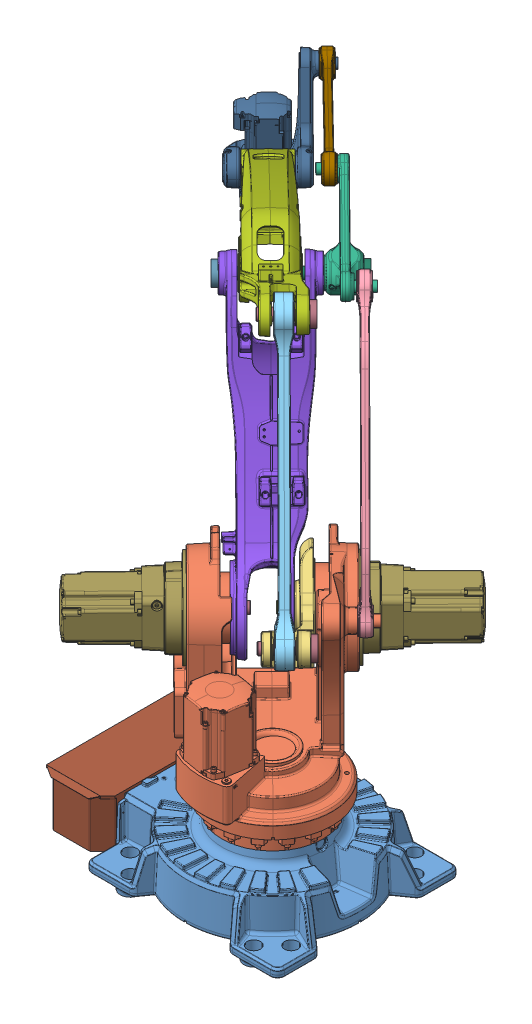
SolidWorks assembly 装配体, configuration 默认. Lengths in mm.
Overall size (188.36 192.9 189.31).
24 component instances, 20 part files, 53 mates.
Components (placement in the parent):
- 111-1: 111 [Default] at (31.9169 -93.0773 0.0393) size (77.8 26.1 72.28)
- 222-1: 222 [Default] at (108.2572 -470.9107 80.6307) x (-0.711585 0 -0.7026) z (0.7026 0 -0.711585) size (72.42 79.23 57.6)
- 333-1: 333 [Default] at (-54.6427 48.8539 -123.2904) x (0.674502 0.318604 0.665987) z (-0.7026 0 0.711585) size (59.48 34.02 15.46)
- 444-1: 444 [Default] at (139.3919 -302.9342 96.1752) x (-0.640122 -0.436772 -0.63204) z (0.7026 0 -0.711585) size (13.8 104.1 4.57)
- 555-1: 555 [Default] at (149.2261 -292.6873 136.4449) x (0.640122 0.436772 0.63204) z (-0.7026 0 0.711585) size (12.5 107 6.85)
- 666-1: 666 [Default] at (-33.4489 78.7584 -68.0821) x (0.700774 -0.173648 0.691926) z (-0.7026 0 0.711585) size (58.22 29.07 16.9)
- 777-2: 777 [Default] at (110.2288 184.9276 106.6261) x (0.7026 0 -0.711585) z (0.674502 0.318604 0.665987) size (19.78 28.14 154.01)
- 888-1: 888 [Default] at (110.474 -208.6533 84.8633) x (-0.640122 -0.436772 -0.63204) z (0.7026 0 -0.711585) size (35.62 116.33 33.14)
- 999-1: 999 [Default] at (261.0446 326.7026 228.677) x (0.226714 -0.947888 0.223851) z (0.7026 0 -0.711585) size (9.6 112.1 5.52)
- 100-1: 100 [默认] at (759.4438 355.8144 743.7493) x (0.7026 0 -0.711585) z (0.711585 0 0.7026) size (32.4 48.93 38.5)
- 1111-1: 1111 [Default] at (482.4826 -100.5846 -7.6891) size (25.2 20.1 57.39)
- 电机-1: 电机 [Default] at (107.7654 -470.9107 81.1289) x (-0.711585 0 -0.7026) z (0.7026 0 -0.711585) size (32.5 32.5 40.6)
- 电机-2: 电机 [Default] at (-132.1184 -470.9107 -117.9487) x (0.711585 0 0.7026) z (-0.7026 0 0.711585) size (32.5 32.5 40.6)
- 销轴1-1: 销轴1 [默认] at (22.1458 89.8559 0.7935) x (0.711585 0 0.7026) z (-0.7026 0 0.711585) size (8 8 17)
- 销轴1-2: 销轴1 [默认] at (-7.2775 174.8655 -28.1529) x (0.711585 0 0.7026) z (-0.7026 0 0.711585) size (8 8 17)
- 销轴2-1: 销轴2 [默认] at (-52.0159 162.1213 -36.8071) x (-0.711585 0 -0.7026) z (0.7026 0 -0.711585) size (8 8 13)
- 销轴3-1: 销轴3 [默认] at (-23.4903 162.1213 -65.6974) x (0.711585 0 0.7026) z (-0.7026 0 0.711585) size (8 8 25)
- 销轴1-3: 销轴1 [默认] at (-27.0014 77.1117 -3.3955) x (-0.022337 0.999507 -0.022055) z (0.7026 0 -0.711585) size (8 8 17)
- 销轴4-1: 销轴4 [默认] at (2.6483 77.1117 -33.4244) x (0.711585 0 0.7026) z (-0.7026 0 0.711585) size (8 8 22)
- 零件21-1: 零件21 [默认] at (31.9169 8.1617 0.0393) x (-1 0 0) z (0 1 0)
- 零件22-1: 零件22 [默认] at origin
- 零件23-1: 零件23 [默认] at origin
- 销轴5-1: 销轴5 [默认] at (-113.9156 129.4644 -112.4) x (0.711585 0 0.7026) z (-0.7026 0 0.711585) size (4 4 8.5)
- 销轴5-2: 销轴5 [默认] at (-102.0416 129.4644 -124.4258) x (0.711585 0 0.7026) z (-0.7026 0 0.711585) size (4 4 8.5)
Mates (geometry in assembly coordinates):
- 重合1: coincident anti-aligned: plane of 111-1 through (23.1842 26.4117 0) normal (0 1 0); plane of 222-1 through (18.2811 26.4117 11.9442) normal (0 -1 0)
- 距离4: distance = 6.45 mm aligned: plane of 777-2 through (-7.2775 174.8655 -28.1529) normal (0.7026 0 -0.711585); plane of 555-1 through (-11.8093 174.8655 -23.5632) normal (0.7026 0 -0.711585)
- 距离5: distance = 16.5 mm anti-aligned: plane of 888-1 through (-17.5163 77.1117 -13.0019) normal (0.7026 0 -0.711585); plane of 222-1 through (-29.1092 77.1117 -1.2607) normal (-0.7026 0 0.711585)
- 宽度2: width aligned: plane of 1111-1 through (-37.6535 4.5617 28.3619) normal (0 0 1); plane of 1111-1 through (-37.6535 22.3617 -28.3619) normal (0 0 -1); plane of 111-1 through (-31.711 8.1617 20.8505) normal (0 0.052336 0.99863); plane of 111-1 through (-25.55 8.1617 -20.8505) normal (0 0.052336 -0.99863)
- 同心13: concentric aligned: cylinder of 222-1 through (23.1833 91.1959 -16.5214) axis (0.7026 0 -0.711585) radius 2; cylinder of 444-1 through (19.5298 91.1959 -12.8211) axis (0.7026 0 -0.711585) radius 2.25
- 同心14: concentric aligned: cylinder of 333-1 through (12.5265 89.8559 10.5357) axis (0.7026 0 -0.711585) radius 2; cylinder of 555-1 through (4.4094 89.8559 18.7566) axis (0.7026 0 -0.711585) radius 2.25
- 宽度3: width anti-aligned: plane of 333-1 through (-46.9472 200.689 -62.2977) normal (-0.7026 0 0.711585); plane of 333-1 through (-16.9048 75.3142 -22.3056) normal (0.7026 0 -0.711585); plane of 555-1 through (18.9665 89.8559 4.0134) normal (0.7026 0 -0.711585); plane of 555-1 through (15.0319 89.8559 7.9983) normal (-0.7026 0 0.711585)
- 同心15: concentric aligned: cylinder of 333-1 through (12.5265 89.8559 10.5357) axis (0.7026 0 -0.711585) radius 2; cylinder of 销轴1-1 through (11.6067 89.8559 11.4672) axis (0.7026 0 -0.711585) radius 2
- 重合16: coincident anti-aligned: plane of 333-1 through (28.8056 77.7045 7.3692) normal (0.7026 0 -0.711585); plane of 销轴1-1 through (22.1458 89.8559 0.7935) normal (-0.7026 0 0.711585)
- 同心16: concentric aligned: cylinder of 555-1 through (-24.1632 174.8655 -11.0514) axis (0.7026 0 -0.711585) radius 2.25; cylinder of 777-2 through (-19.7388 174.8655 -15.5324) axis (0.7026 0 -0.711585) radius 2
- 同心17: concentric aligned: cylinder of 777-2 through (-19.7388 174.8655 -15.5324) axis (0.7026 0 -0.711585) radius 2; cylinder of 销轴1-2 through (-17.8166 174.8655 -17.4792) axis (0.7026 0 -0.711585) radius 2
- 重合17: coincident anti-aligned: plane of 777-2 through (-7.2775 174.8655 -28.1529) normal (0.7026 0 -0.711585); plane of 销轴1-2 through (-7.2775 174.8655 -28.1529) normal (-0.7026 0 0.711585)
- 同心18: concentric aligned: cylinder of 444-1 through (-6.2135 176.2055 -45.4946) axis (0.7026 0 -0.711585) radius 2; cylinder of 666-1 through (-14.3271 176.2055 -37.2773) axis (0.7026 0 -0.711585) radius 1.75
- 同心19: concentric aligned: cylinder of 777-2 through (-55.6504 162.1213 -33.1261) axis (0.7026 0 -0.711585) radius 2.25; cylinder of 888-1 through (-63.5848 162.1213 -25.0902) axis (0.7026 0 -0.711585) radius 2
- 同心20: concentric aligned: cylinder of 777-2 through (-27.9708 162.1213 -61.1597) axis (-0.7026 0 0.711585) radius 2.25; cylinder of 888-1 through (-19.7904 162.1213 -69.4446) axis (-0.7026 0 0.711585) radius 2
- 同心21: concentric anti-aligned: cylinder of 666-1 through (-39.987 162.1213 -48.9898) axis (0.7026 0 -0.711585) radius 2.25; cylinder of 888-1 through (-19.7904 162.1213 -69.4446) axis (-0.7026 0 0.711585) radius 2
- 同心22: concentric anti-aligned: cylinder of 销轴2-1 through (-44.2873 162.1213 -44.6345) axis (-0.7026 0 0.711585) radius 2; cylinder of 888-1 through (-63.5848 162.1213 -25.0902) axis (0.7026 0 -0.711585) radius 2
- 重合18: coincident anti-aligned: plane of 888-1 through (-52.0159 162.1213 -36.8071) normal (-0.7026 0 0.711585); plane of 销轴2-1 through (-52.0159 162.1213 -36.8071) normal (0.7026 0 -0.711585)
- 同心23: concentric aligned: cylinder of 666-1 through (-39.987 162.1213 -48.9898) axis (0.7026 0 -0.711585) radius 2.25; cylinder of 销轴3-1 through (-39.6501 162.1213 -49.331) axis (0.7026 0 -0.711585) radius 2
- 重合19: coincident anti-aligned: plane of 666-1 through (-23.4903 162.1213 -65.6974) normal (0.7026 0 -0.711585); plane of 销轴3-1 through (-23.4903 162.1213 -65.6974) normal (-0.7026 0 0.711585)
- 同心25: concentric aligned: cylinder of 222-1 through (-31.498 77.1117 1.1586) axis (0.7026 0 -0.711585) radius 2; cylinder of 333-1 through (-10.8767 77.1117 -19.7264) axis (0.7026 0 -0.711585) radius 2.25
- 距离7: distance = 5.85 mm aligned: plane of 333-1 through (-6.8016 77.1117 -23.8536) normal (-0.7026 0 0.711585); plane of 222-1 through (-2.6914 77.1117 -28.0163) normal (-0.7026 0 0.711585)
- 重合21: coincident anti-aligned: plane of 222-1 through (-27.0014 77.1117 -3.3955) normal (-0.7026 0 0.711585); plane of 销轴1-3 through (-27.0014 77.1117 -3.3955) normal (0.7026 0 -0.711585)
- 同心27: concentric aligned: cylinder of 222-1 through (-31.498 77.1117 1.1586) axis (0.7026 0 -0.711585) radius 2; cylinder of 销轴4-1 through (-11.4037 77.1117 -19.1927) axis (0.7026 0 -0.711585) radius 2
- 重合22: coincident anti-aligned: plane of 222-1 through (2.6483 77.1117 -33.4244) normal (0.7026 0 -0.711585); plane of 销轴4-1 through (2.6483 77.1117 -33.4244) normal (-0.7026 0 0.711585)
- 同心28: concentric aligned: cylinder of 222-1 through (-24.191 87.1117 -6.2418) axis (-0.7026 0 0.711585) radius 1.75; cylinder of 电机-1 through (-25.3854 87.1117 -5.0321) axis (-0.7026 0 0.711585) radius 1.75
- 同心30: concentric aligned: cylinder of 电机-2 through (1.0324 87.1117 -31.7877) axis (0.7026 0 -0.711585) radius 1.75; cylinder of 222-1 through (-0.1621 87.1117 -30.578) axis (0.7026 0 -0.711585) radius 1.75
- 距离8: distance = 0.675 mm anti-aligned: plane of 100-1 through (-105.2033 129.4644 -121.2237) normal (-0.7026 0 0.711585); plane of 777-2 through (-105.6776 129.4644 -120.7434) normal (0.7026 0 -0.711585)
- 同心33: concentric anti-aligned: cylinder of 999-1 through (-108.0666 148.748 -151.0328) axis (-0.7026 0 0.711585) radius 2; cylinder of 100-1 through (-111.4022 148.748 -147.6545) axis (0.7026 0 -0.711585) radius 1.75
- 距离9: distance = 7.95 mm anti-aligned: plane of 999-1 through (-61.4728 206.1243 -90.6228) normal (0.7026 0 -0.711585); plane of 100-1 through (-119.8205 125.9644 -137.0616) normal (-0.7026 0 0.711585)
- 同心34: concentric aligned: cylinder of 666-1 through (-37.6055 181.4049 -84.1107) axis (-0.7026 0 0.711585) radius 1.75; cylinder of 999-1 through (-41.2487 181.4049 -80.421) axis (-0.7026 0 0.711585) radius 2
- 重合25: coincident anti-aligned: plane of 222-1 through (23.1833 91.1959 -16.5214) normal (0.7026 0 -0.711585); plane of 444-1 through (23.1833 91.1959 -16.5214) normal (-0.7026 0 0.711585)
- 在位1: in place: line of 111-1 through (37.9183 8.1617 24.3505) axis (0 1 0); plane of ? through (0 8.1617 0) normal (0 1 0); moOrthogonalPlaneRef_w of 111-1 through (37.9183 8.1617 24.3505) axis (0 1 0); unknown of ?; line of 111-1 through (37.9183 8.1617 24.3505) axis (0 1 0); line of ? through (-55 0 8.1617) axis (0 -1 0); plane of 111-1 through (37.9183 8.1617 24.3505) normal (0 1 0); unknown of 零件21-1
- 重合26: coincident aligned: plane of 111-1; plane of 零件21-1
- 重合27: coincident aligned: moOrthogonalPlaneRef_w of 111-1 through (31.9169 8.1617 0.0393) axis (0 0 1); plane of 零件21-1 through (0 -1000 0) normal (0 0 1)
- 重合28: coincident anti-aligned: moOrthogonalPlaneRef_w of 111-1 through (31.9169 8.1617 0.0393) axis (1 0 0); plane of 零件21-1
- 同心35: concentric anti-aligned: cylinder of 111-1 through (6.1842 2.9617 0) axis (0 1 0) radius 4; cylinder of 222-1 through (6.1842 18.8617 0) axis (0 -1 0) radius 1.65
- 重合29: coincident anti-aligned: plane of 666-1 through (-44.926 184.0147 -76.0416) normal (-0.7026 0 0.711585); plane of 999-1 through (-45.2535 181.4049 -76.3649) normal (0.7026 0 -0.711585)
- 同心36: concentric anti-aligned: cylinder of 222-1 through (-31.498 77.1117 1.1586) axis (0.7026 0 -0.711585) radius 2; cylinder of 销轴1-3 through (-16.4624 77.1117 -14.0693) axis (-0.7026 0 0.711585) radius 2
- 同心37: concentric aligned: cylinder of 222-1 through (-0.1621 67.1117 -30.578) axis (0.7026 0 -0.711585) radius 1.75; cylinder of 电机-2 through (1.0324 67.1117 -31.7877) axis (0.7026 0 -0.711585) radius 1.75
- 同心38: concentric aligned: cylinder of 222-1 through (-24.191 67.1117 -6.2418) axis (-0.7026 0 0.711585) radius 1.75; cylinder of 电机-1 through (-25.3854 67.1117 -5.0321) axis (-0.7026 0 0.711585) radius 1.75
- 同心39: concentric aligned: cylinder of 888-1 through (-11.4037 77.1117 -19.1927) axis (0.7026 0 -0.711585) radius 2.25; cylinder of 销轴4-1 through (-11.4037 77.1117 -19.1927) axis (0.7026 0 -0.711585) radius 2
- 同心41: concentric aligned: cylinder of 111-1 through (-31.3158 17.4617 21.4) axis (-1 0 0) radius 1; cylinder of 1111-1 through (-31.3158 17.4617 21.4) axis (-1 0 0) radius 1
- 同心42: concentric aligned: cylinder of 111-1 through (-31.3158 9.4617 21.4) axis (-1 0 0) radius 1; cylinder of 1111-1 through (-31.3158 9.4617 21.4) axis (-1 0 0) radius 1
- 重合33: coincident anti-aligned: plane of 111-1 through (-32.3158 25.7746 -18.4) normal (-1 0 0); plane of 1111-1 through (-32.3158 77.4617 24.6903) normal (1 0 0)
- 重合35: coincident anti-aligned: plane of 222-1 through (-29.1092 77.1117 -1.2607) normal (-0.7026 0 0.711585); plane of 电机-1 through (-29.1092 77.1117 -1.2607) normal (0.7026 0 -0.711585)
- 重合36: coincident anti-aligned: plane of 222-1 through (4.7562 77.1117 -35.5591) normal (0.7026 0 -0.711585); plane of 电机-2 through (4.7562 77.1117 -35.5591) normal (-0.7026 0 0.711585)
- 同心43: concentric anti-aligned: cylinder of 777-2 through (-117.2585 129.4644 -109.0144) axis (0.7026 0 -0.711585) radius 2; circle of 100-1
- 同心44: concentric aligned: cylinder of 777-2 through (-117.2585 129.4644 -109.0144) axis (0.7026 0 -0.711585) radius 2; cylinder of 100-1 through (-119.8877 129.4644 -106.3515) axis (0.7026 0 -0.711585) radius 2.25
- 重合37: coincident aligned: plane of 100-1 through (-119.8877 129.4644 -106.3516) normal (-0.7026 0 0.711585); plane of 销轴5-1 through (-119.8877 129.4644 -106.3516) normal (-0.7026 0 0.711585)
- 同心45: concentric aligned: cylinder of 100-1 through (-119.8877 129.4644 -106.3515) axis (0.7026 0 -0.711585) radius 2.25; cylinder of 销轴5-1 through (-119.8877 129.4644 -106.3516) axis (0.7026 0 -0.711585) radius 2
- 同心46: concentric aligned: cylinder of 777-2 through (-117.2585 129.4644 -109.0144) axis (0.7026 0 -0.711585) radius 2; cylinder of 销轴5-2 through (-108.0137 129.4644 -118.3774) axis (0.7026 0 -0.711585) radius 2
- 重合38: coincident aligned: plane of 100-1 through (-102.0416 129.4644 -124.4258) normal (0.7026 0 -0.711585); plane of 销轴5-2 through (-102.0416 129.4644 -124.4258) normal (0.7026 0 -0.711585)
